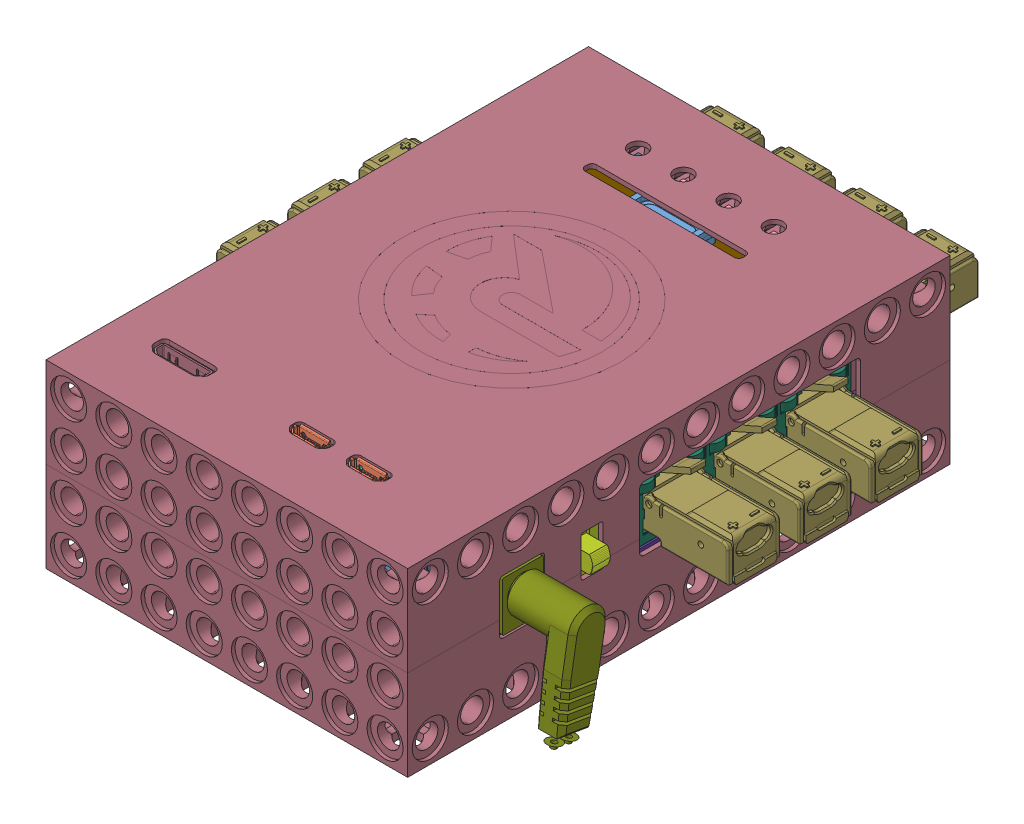
SolidWorks assembly PCBA_estimation_20190215, configuration Default. Lengths in mm.
Overall size (114.3 40.23 137.41).
1046 component instances, 72 part files, 0 mates.
Components (placement in the parent):
- RapberryPiZero-1: RapberryPiZero [Default] at (82.9427 2.6354 70.9883) x (1 0 0) z (0 1 0) size (66.85 4.45 31.23)
  - Raspberry_pizero_PCB-1: Raspberry_pizero_PCB [Default] at (-51.2564 20.0966 13.0542) size (65 1 30)
  - Micro USB_input_female (short)-SMT-1: Micro USB_input_female (short)-SMT [Default] at (-29.7564 22.3216 26.5042) size (7.98 2.94 5.43)
  - Micro USB_input_female (short)-SMT-2: Micro USB_input_female (short)-SMT [Default] at (-42.3564 22.3216 26.5042) size (7.98 2.94 5.43)
  - 0204 - Capacitor-1: 0204 - Capacitor [Default] at (-60.0807 21.3466 22.3712) x (0 0 -1) z (1 0 0) size (1.08 0.58 0.68)
  - 0204 - Capacitor-2: 0204 - Capacitor [Default] at (-43.6156 21.3466 13.1418) size (1.08 0.58 0.68)
  - 0204 - Capacitor-3: 0204 - Capacitor [Default] at (-62.4121 21.3466 11.2398) size (1.08 0.58 0.68)
  - 0204 - Capacitor-4: 0204 - Capacitor [Default] at (-45.7322 21.3466 20.0663) size (1.08 0.58 0.68)
  - 0204 - Capacitor-5: 0204 - Capacitor [Default] at (-43.6156 21.3466 10.1424) size (1.08 0.58 0.68)
  - 0204 - Capacitor-6: 0204 - Capacitor [Default] at (-59.0466 21.3466 22.3712) x (0 0 -1) z (1 0 0) size (1.08 0.58 0.68)
  - 0204 - Capacitor-7: 0204 - Capacitor [Default] at (-46.3457 21.3466 16.1412) size (1.08 0.58 0.68)
  - 0204 - Capacitor-8: 0204 - Capacitor [Default] at (-48.9117 21.3466 7.6917) size (1.08 0.58 0.68)
  - 0204 - Capacitor-9: 0204 - Capacitor [Default] at (-62.5919 21.3466 21.919) size (1.08 0.58 0.68)
  - 0204 - Capacitor-10: 0204 - Capacitor [Default] at (-48.1448 21.3466 22.316) x (0 0 -1) z (1 0 0) size (1.08 0.58 0.68)
  - 0204 - Capacitor-11: 0204 - Capacitor [Default] at (-55.4926 21.3466 7.2526) x (0 0 -1) z (1 0 0) size (1.08 0.58 0.68)
  - 0204 - Capacitor-12: 0204 - Capacitor [Default] at (-52.6496 21.3466 22.316) x (0 0 1) z (-1 0 0) size (1.08 0.58 0.68)
  - 0204 - Capacitor-13: 0204 - Capacitor [Default] at (-53.7932 21.3466 7.2526) x (0 0 1) z (-1 0 0) size (1.08 0.58 0.68)
  - 0204 - Capacitor-14: 0204 - Capacitor [Default] at (-61.8122 21.3466 17.2416) size (1.08 0.58 0.68)
  - 0204 - Capacitor-15: 0204 - Capacitor [Default] at (-45.7322 21.3466 19.0675) size (1.08 0.58 0.68)
  - 0204 - Capacitor-16: 0204 - Capacitor [Default] at (-60.4584 21.3466 22.3712) x (0 0 1) z (-1 0 0) size (1.08 0.58 0.68)
  - 0204 - Capacitor-17: 0204 - Capacitor [Default] at (-45.7322 21.3466 17.1095) size (1.08 0.58 0.68)
  - 0204 - Capacitor-18: 0204 - Capacitor [Default] at (-46.475 21.3466 21.113) size (1.08 0.58 0.68)
  - 0204 - Capacitor-19: 0204 - Capacitor [Default] at (-59.8477 21.3466 7.2526) x (0 0 1) z (-1 0 0) size (1.08 0.58 0.68)
  - 0204 - Capacitor-20: 0204 - Capacitor [Default] at (-46.3457 21.3466 15.1229) size (1.08 0.58 0.68)
  - 0204 - Capacitor-21: 0204 - Capacitor [Default] at (-45.7322 21.3466 18.1249) size (1.08 0.58 0.68)
  - 0204 - Capacitor-22: 0204 - Capacitor [Default] at (-51.2398 21.3466 22.316) x (0 0 -1) z (1 0 0) size (1.08 0.58 0.68)
  - 0204 - Capacitor-23: 0204 - Capacitor [Default] at (-47.1199 21.3466 23.926) x (0 0 1) z (-1 0 0) size (1.08 0.58 0.68)
  - 0204 - Capacitor-24: 0204 - Capacitor [Default] at (-62.4121 21.3466 12.2528) size (1.08 0.58 0.68)
  - 0204 - Capacitor-25: 0204 - Capacitor [Default] at (-48.9117 21.3466 6.5273) size (1.08 0.58 0.68)
  - 0204 - Capacitor-26: 0204 - Capacitor [Default] at (-61.8122 21.3466 13.3136) size (1.08 0.58 0.68)
  - 0204 - Capacitor-27: 0204 - Capacitor [Default] at (-61.8122 21.3466 15.241) size (1.08 0.58 0.68)
  - 0204 - Capacitor-28: 0204 - Capacitor [Default] at (-61.8122 21.3466 14.2646) size (1.08 0.58 0.68)
  - 0204 - Capacitor-29: 0204 - Capacitor [Default] at (-46.3457 21.3466 14.0197) size (1.08 0.58 0.68)
  - 0204 - Capacitor-30: 0204 - Capacitor [Default] at (-62.5919 21.3466 20.9695) size (1.08 0.58 0.68)
  - 0204 - Capacitor-31: 0204 - Capacitor [Default] at (-52.25 21.3466 22.316) x (0 0 -1) z (1 0 0) size (1.08 0.58 0.68)
  - 0204 - Capacitor-32: 0204 - Capacitor [Default] at (-61.8122 21.3466 16.2144) size (1.08 0.58 0.68)
  - 0204 - Capacitor-33: 0204 - Capacitor [Default] at (-46.3457 21.3466 12.9589) size (1.08 0.58 0.68)
  - 0204 - Capacitor-34: 0204 - Capacitor [Default] at (-49.1841 21.3466 22.316) x (0 0 -1) z (1 0 0) size (1.08 0.58 0.68)
  - 0204- Resistor-1: 0204- Resistor [Default] at (-61.8169 21.4522 19.8533) x (-1 0 0) z (0 -1 0) size (0.99 0.51 0.36)
  - 0204- Resistor-2: 0204- Resistor [Default] at (-43.6109 21.4522 15.4193) x (-1 0 0) z (0 -1 0) size (0.99 0.51 0.36)
  - 0204- Resistor-3: 0204- Resistor [Default] at (-65.0626 21.4522 16.5355) x (1 0 0) z (0 -1 0) size (0.99 0.51 0.36)
  - 0204- Resistor-4: 0204- Resistor [Default] at (-42.6936 21.4522 18.4076) x (-1 0 0) z (0 -1 0) size (0.99 0.51 0.36)
  - 0204- Resistor-5: 0204- Resistor [Default] at (-61.8169 21.4522 18.5178) x (-1 0 0) z (0 -1 0) size (0.99 0.51 0.36)
  - 0204- Resistor-6: 0204- Resistor [Default] at (-79.148 21.4522 17.7279) x (-1 0 0) z (0 -1 0) size (0.99 0.51 0.36)
  - 0204- Resistor-7: 0204- Resistor [Default] at (-39.831 21.4522 18.1462) x (0 0 1) z (0 -1 0) size (0.99 0.51 0.36)
  - 0204- Resistor-8: 0204- Resistor [Default] at (-78.9105 21.4522 21.1554) x (1 0 0) z (0 -1 0) size (0.99 0.51 0.36)
  - 0204- Resistor-9: 0204- Resistor [Default] at (-43.6109 21.4522 14.4127) x (-1 0 0) z (0 -1 0) size (0.99 0.51 0.36)
  - 0204- Resistor-10: 0204- Resistor [Default] at (-52.4165 21.4522 24.0419) x (1 0 0) z (0 -1 0) size (0.99 0.51 0.36)
  - 0204- Resistor-11: 0204- Resistor [Default] at (-43.6109 21.4522 12.4047) x (-1 0 0) z (0 -1 0) size (0.99 0.51 0.36)
  - 0204- Resistor-12: 0204- Resistor [Default] at (-68.4329 21.4522 5.4384) x (0 0 1) z (0 -1 0) size (0.99 0.51 0.36)
  - 0204- Resistor-13: 0204- Resistor [Default] at (-21.8613 21.4522 20.9026) x (-1 0 0) z (0 -1 0) size (0.99 0.51 0.36)
  - 0204- Resistor-14: 0204- Resistor [Default] at (-69.7255 21.4522 5.4384) x (0 0 1) z (0 -1 0) size (0.99 0.51 0.36)
  - 0204- Resistor-15: 0204- Resistor [Default] at (-56.0985 21.4522 7.2479) x (0 0 -1) z (0 -1 0) size (0.99 0.51 0.36)
  - 0204- Resistor-16: 0204- Resistor [Default] at (-48.8769 21.4522 23.8207) x (1 0 0) z (0 -1 0) size (0.99 0.51 0.36)
  - 0204- Resistor-17: 0204- Resistor [Default] at (-28.0827 21.4522 9.5819) x (-1 0 0) z (0 -1 0) size (0.99 0.51 0.36)
  - CAP-0306-1: CAP-0306 [Default] at (-45.8903 21.4966 8.7634) size (1.6 0.8 0.9)
  - CAP-0306-2: CAP-0306 [Default] at (-82.0031 21.4966 19.0464) x (0 0 1) z (-1 0 0) size (1.6 0.8 0.9)
  - Raspberry_pizero_BCM2835 with VC4-1: Raspberry_pizero_BCM2835 with VC4 [Default] at (-54.1608 21.5466 15.1238) x (1 0 0) z (0 0 -1) size (12 0.65 12)
  - Crystal 3.4x2.4mm-1: Crystal 3.4x2.4mm [Default] at (-65.3089 21.0966 19.2633) size (3.2 1 2.4)
  - 32,768 Khz Crystal-1: 32,768 Khz Crystal [Default] at (-60.5154 21.1428 26.5473) x (0.999848 -0.017452 0) z (0 0 1) size (3.4 1.03 1.5)
  - 0805- Capacitor-1: 0805- Capacitor [Default] at (-27.9052 21.9966 13.3538) x (0 0 -1) z (0 -1 0) size (2 1.25 0.9)
  - 0805- Capacitor-2: 0805- Capacitor [Default] at (-29.8247 21.9966 13.3538) x (0 0 1) z (0 -1 0) size (2 1.25 0.9)
  - 0805- Capacitor-3: 0805- Capacitor [Default] at (-20.9924 21.9966 13.3538) x (0 0 -1) z (0 -1 0) size (2 1.25 0.9)
  - 0805- Capacitor-4: 0805- Capacitor [Default] at (-51.9496 21.9966 7.3589) x (1 0 0) z (0 -1 0) size (2 1.25 0.9)
  - 0805- Capacitor-5: 0805- Capacitor [Default] at (-37.009 21.9966 22.5384) x (0 0 -1) z (0 -1 0) size (2 1.25 0.9)
  - 0805- Capacitor-6: 0805- Capacitor [Default] at (-51.9496 21.9966 5.2384) x (1 0 0) z (0 -1 0) size (2 1.25 0.9)
  - 0805- Capacitor-7: 0805- Capacitor [Default] at (-22.8003 21.9966 13.3538) x (0 0 -1) z (0 -1 0) size (2 1.25 0.9)
  - 0204 - Capacitor Brown-1: 0204 - Capacitor Brown [Default] at (-28.0874 21.3466 10.3236) size (1.08 0.58 0.68)
  - 0204 - Capacitor Brown-2: 0204 - Capacitor Brown [Default] at (-46.3457 21.3466 10.1566) size (1.08 0.58 0.68)
  - 0204 - Capacitor Brown-3: 0204 - Capacitor Brown [Default] at (-43.6156 21.3466 11.1151) size (1.08 0.58 0.68)
  - 0204 - Capacitor Brown-4: 0204 - Capacitor Brown [Default] at (-64.0312 21.3466 26.8794) size (1.08 0.58 0.68)
  - 0204 - Capacitor Brown-5: 0204 - Capacitor Brown [Default] at (-46.3457 21.3466 11.0963) size (1.08 0.58 0.68)
  - 0204 - Capacitor Brown-6: 0204 - Capacitor Brown [Default] at (-57.5817 21.3466 26.803) size (1.08 0.58 0.68)
  - 0204 - Capacitor Brown-7: 0204 - Capacitor Brown [Default] at (-46.3457 21.3466 12.214) size (1.08 0.58 0.68)
  - 0204 - Capacitor Brown-8: 0204 - Capacitor Brown [Default] at (-80.6197 21.3466 20.6997) size (1.08 0.58 0.68)
  - 6-Pin SOT-1: 6-Pin SOT [Default] at (-79.714 21.0966 19.2138) x (0 0 1) z (0 1 0) size (1.5 1.84 0.95)
  - micro sd molex-1: micro sd molex [Default] at (-74.7768 21.6766 -33.0961) x (0 0 1) z (0 1 0) size (11.95 11.4 1.45)
  - hdmi type C-1: hdmi type C [Default] at (-71.3564 22.9466 28.6542) size (12.9 4.05 7.7)
  - Voltage Regulator 3x3mm 12-Pin-1: Voltage Regulator 3x3mm 12-Pin [Default] at (-23.6842 21.0966 12.6105) x (1 0 0) z (0 1 0) size (3 4.1 1.28)
  - 1210 inductor-1: 1210 inductor [Default] at (-46.4963 21.0916 6.3909) x (0 0 1) z (0 1 0) size (3.43 2.77 0.72)
  - 1210 inductor-2: 1210 inductor [Default] at (-28.2854 21.0916 17.6682) x (1 0 0) z (0 1 0) size (3.43 2.77 0.72)
  - 1210 inductor-3: 1210 inductor [Default] at (-22.7405 21.0916 9.2394) x (1 0 0) z (0 1 0) size (3.43 2.77 0.72)
  - 545482271-1: 545482271 [Default] at (-21.4564 21.1166 13.0542) x (0 0 -1) z (1 0 0) size (16.2 1.2 5)
- RRRC_carrier_board-1: RRRC_carrier_board [Default] at (75.1836 8.28 47.3515) x (0 0 -1) z (0 1 0) size (102.74 81.4 21.81)
  - Board_CARRIER_3-1: Board_CARRIER_3 [Default] at origin size (102.7 77 1.61)
    - Open CASCADE STEP translator 6.8 1.1.1_2-1: Open CASCADE STEP translator 6.8 1.1.1_2 [Default] at (0 0 -1.61) size (102.7 77 1.61)
  - D59_CARRIER_3-1: D59_CARRIER_3 [Default] at origin size (0.65 1.05 0.44)
    - SOD-923_3-1: SOD-923_3 [Default] at (80 52.05 0) x (0 1 0) z (1 0 0) size (1.05 0.44 0.65)
  - D15_CARRIER_3-1: D15_CARRIER_3 [Default] at origin size (1.7 1.7 0.64)
    - SOT-666_3-1: SOT-666_3 [Default] at (15.825 38.45 0) x (1 0 0) z (0 0 1) size (1.7 1.7 0.64)
  - C71_CARRIER_3-1: C71_CARRIER_3 [Default] at origin size (1 0.5 0.5)
    - C_0402_3-1: C_0402_3 [Default] at (44.4 57.5 0) x (-1 0 0) z (0 0 1) size (1 0.5 0.5)
  - D71_CARRIER_3-1: D71_CARRIER_3 [Default] at origin size (1.05 0.65 0.44)
    - SOD-923_3-1: SOD-923_3 [Default] at (62.45 58.75 0) x (-1 0 0) z (0 1 0) size (1.05 0.44 0.65)
  - D70_CARRIER_3-1: D70_CARRIER_3 [Default] at origin size (1.05 0.65 0.44)
    - SOD-923_3-1: SOD-923_3 [Default] at (66.95 57.6 0) x (1 0 0) z (0 -1 0) size (1.05 0.44 0.65)
  - D69_CARRIER_3-1: D69_CARRIER_3 [Default] at origin size (1.05 0.65 0.44)
    - SOD-923_3-1: SOD-923_3 [Default] at (50.1 57.5 0) x (1 0 0) z (0 -1 0) size (1.05 0.44 0.65)
  - D68_CARRIER_3-1: D68_CARRIER_3 [Default] at origin size (1.05 0.65 0.44)
    - SOD-923_3-1: SOD-923_3 [Default] at (52.85 58.45 0) x (-1 0 0) z (0 1 0) size (1.05 0.44 0.65)
  - D67_CARRIER_3-1: D67_CARRIER_3 [Default] at origin size (1.05 0.65 0.44)
    - SOD-923_3-1: SOD-923_3 [Default] at (37.65 58.6 0) x (1 0 0) z (0 -1 0) size (1.05 0.44 0.65)
  - D66_CARRIER_3-1: D66_CARRIER_3 [Default] at origin size (1.05 0.65 0.44)
    - SOD-923_3-1: SOD-923_3 [Default] at (44.35 58.55 0) x (-1 0 0) z (0 1 0) size (1.05 0.44 0.65)
  - D65_CARRIER_3-1: D65_CARRIER_3 [Default] at origin size (1.05 0.65 0.44)
    - SOD-923_3-1: SOD-923_3 [Default] at (46.8 18.45 0) x (-1 0 0) z (0 1 0) size (1.05 0.44 0.65)
  - D64_CARRIER_3-1: D64_CARRIER_3 [Default] at origin size (1.05 0.65 0.44)
    - SOD-923_3-1: SOD-923_3 [Default] at (42.85 18.35 0) x (-1 0 0) z (0 1 0) size (1.05 0.44 0.65)
  - D63_CARRIER_3-1: D63_CARRIER_3 [Default] at origin size (1.05 0.65 0.44)
    - SOD-923_3-1: SOD-923_3 [Default] at (60.1 19.2 0) x (1 0 0) z (0 -1 0) size (1.05 0.44 0.65)
  - D62_CARRIER_3-1: D62_CARRIER_3 [Default] at origin size (1.05 0.65 0.44)
    - SOD-923_3-1: SOD-923_3 [Default] at (56.05 18.45 0) x (-1 0 0) z (0 1 0) size (1.05 0.44 0.65)
  - D61_CARRIER_3-1: D61_CARRIER_3 [Default] at origin size (1.05 0.65 0.44)
    - SOD-923_3-1: SOD-923_3 [Default] at (73.3 18.5 0) x (-1 0 0) z (0 1 0) size (1.05 0.44 0.65)
  - D60_CARRIER_3-1: D60_CARRIER_3 [Default] at origin size (1.05 0.65 0.44)
    - SOD-923_3-1: SOD-923_3 [Default] at (69.4 18.5 0) x (-1 0 0) z (0 1 0) size (1.05 0.44 0.65)
  - D11_CARRIER_3-1: D11_CARRIER_3 [Default] at origin size (1.15 0.55 0.41)
    - R_0402_3-1: R_0402_3 [Default] at (48.775 25.425 0) x (1 0 0) z (0 -1 0) size (1.15 0.41 0.55)
  - R99_CARRIER_3-1: R99_CARRIER_3 [Default] at origin size (1.15 0.55 0.41)
    - R_0402_3-1: R_0402_3 [Default] at (83.975 18.15 0) x (-1 0 0) z (0 1 0) size (1.15 0.41 0.55)
  - D58_CARRIER_3-1: D58_CARRIER_3 [Default] at origin size (1.05 0.65 0.44)
    - SOD-923_3-1: SOD-923_3 [Default] at (78.05 20.3 0) x (-1 0 0) z (0 1 0) size (1.05 0.44 0.65)
  - D57_CARRIER_3-1: D57_CARRIER_3 [Default] at origin size (0.65 1.05 0.44)
    - SOD-923_3-1: SOD-923_3 [Default] at (79.85 30.3 0) x (0 1 0) z (1 0 0) size (1.05 0.44 0.65)
  - D56_CARRIER_3-1: D56_CARRIER_3 [Default] at origin size (0.65 1.05 0.44)
    - SOD-923_3-1: SOD-923_3 [Default] at (79.7 41.4 0) x (0 1 0) z (1 0 0) size (1.05 0.44 0.65)
  - R160_CARRIER_3-1: R160_CARRIER_3 [Default] at origin size (1.15 0.55 0.41)
    - R_0402_3-1: R_0402_3 [Default] at (2.375 14.45 0) x (1 0 0) z (0 -1 0) size (1.15 0.41 0.55)
  - R159_CARRIER_3-1: R159_CARRIER_3 [Default] at origin size (1.15 0.55 0.41)
    - R_0402_3-1: R_0402_3 [Default] at (2.375 15.5 0) x (1 0 0) z (0 -1 0) size (1.15 0.41 0.55)
  - R158_CARRIER_3-1: R158_CARRIER_3 [Default] at origin size (0.55 1.15 0.41)
    - R_0402_3-1: R_0402_3 [Default] at (9.4 16 0) x (0 -1 0) z (-1 0 0) size (1.15 0.41 0.55)
  - Q19_CARRIER_3-1: Q19_CARRIER_3 [Default] at origin size (3.05 3 1.41)
    - SOT95P255X140-3N_3-1: SOT95P255X140-3N_3 [Default] at (5.9 15.45 0) x (0 1 0) z (0 0 1) size (3 3.05 1.41)
  - D24_CARRIER_3-1: D24_CARRIER_3 [Default] at origin size (1.05 0.65 0.44)
    - SOD-923_3-1: SOD-923_3 [Default] at (82.6 28.05 0) x (-1 0 0) z (0 1 0) size (1.05 0.44 0.65)
  - CON1_CARRIER_3-1: CON1_CARRIER_3 [Default] at origin size (6.35 2.14 6.3)
    - SULLINS_GRPB051VWVN-RC_3-1: SULLINS_GRPB051VWVN-RC_3 [Default] at (60.4749 35.8 0) x (1 0 0) z (0 -1 0) size (6.35 6.3 2.14)
  - D54_CARRIER_3-1: D54_CARRIER_3 [Default] at origin size (1.6 3.6 1.3)
    - SOD360X160X130L37X85N_3-1: SOD360X160X130L37X85N_3 [Default] at (57.2 45.75 0) x (0 1 0) z (0 0 1) size (3.6 1.6 1.3)
  - D55_CARRIER_3-1: D55_CARRIER_3 [Default] at origin size (1.6 3.6 1.3)
    - SOD360X160X130L37X85N_3-1: SOD360X160X130L37X85N_3 [Default] at (51.35 45.6 0) x (0 1 0) z (0 0 1) size (3.6 1.6 1.3)
  - Q17_CARRIER_3-1: Q17_CARRIER_3 [Default] at origin size (3.05 3 1.41)
    - SOT95P255X140-3N_3-1: SOT95P255X140-3N_3 [Default] at (54.3 45.7 0) x (0 1 0) z (0 0 1) size (3 3.05 1.41)
  - Q18_CARRIER_3-1: Q18_CARRIER_3 [Default] at origin size (3.05 3 1.41)
    - SOT95P255X140-3N_3-1: SOT95P255X140-3N_3 [Default] at (48.43 45.65 0) x (0 1 0) z (0 0 1) size (3 3.05 1.41)
  - R142_CARRIER_3-1: R142_CARRIER_3 [Default] at origin size (1.15 0.55 0.41)
    - R_0402_3-1: R_0402_3 [Default] at (43.65 48 0) x (-1 0 0) z (0 1 0) size (1.15 0.41 0.55)
  - R144_CARRIER_3-1: R144_CARRIER_3 [Default] at origin size (1.15 0.55 0.41)
    - R_0402_3-1: R_0402_3 [Default] at (49.55 48.1 0) x (1 0 0) z (0 -1 0) size (1.15 0.41 0.55)
  - R147_CARRIER_3-1: R147_CARRIER_3 [Default] at origin size (1.15 0.55 0.41)
    - R_0402_3-1: R_0402_3 [Default] at (48.2 43.2 0) x (-1 0 0) z (0 1 0) size (1.15 0.41 0.55)
  - R139_CARRIER_3-1: R139_CARRIER_3 [Default] at origin size (1.15 0.55 0.41)
    - R_0402_3-1: R_0402_3 [Default] at (48.05 37.2 0) x (-1 0 0) z (0 1 0) size (1.15 0.41 0.55)
  - R135_CARRIER_3-1: R135_CARRIER_3 [Default] at origin size (1.15 0.55 0.41)
    - R_0402_3-1: R_0402_3 [Default] at (48.975 42.1 0) x (1 0 0) z (0 -1 0) size (1.15 0.41 0.55)
  - R133_CARRIER_3-1: R133_CARRIER_3 [Default] at origin size (1.15 0.55 0.41)
    - R_0402_3-1: R_0402_3 [Default] at (43.7 42.15 0) x (-1 0 0) z (0 1 0) size (1.15 0.41 0.55)
  - Q16_CARRIER_3-1: Q16_CARRIER_3 [Default] at origin size (3.05 3 1.41)
    - SOT95P255X140-3N_3-1: SOT95P255X140-3N_3 [Default] at (48.5 39.65 0) x (0 1 0) z (0 0 1) size (3 3.05 1.41)
  - Q15_CARRIER_3-1: Q15_CARRIER_3 [Default] at origin size (3.05 3 1.41)
    - SOT95P255X140-3N_3-1: SOT95P255X140-3N_3 [Default] at (54.35 39.65 0) x (0 1 0) z (0 0 1) size (3 3.05 1.41)
  - D53_CARRIER_3-1: D53_CARRIER_3 [Default] at origin size (1.6 3.6 1.3)
    - SOD360X160X130L37X85N_3-1: SOD360X160X130L37X85N_3 [Default] at (51.425 39.7 0) x (0 1 0) z (0 0 1) size (3.6 1.6 1.3)
  - D52_CARRIER_3-1: D52_CARRIER_3 [Default] at origin size (1.6 3.6 1.3)
    - SOD360X160X130L37X85N_3-1: SOD360X160X130L37X85N_3 [Default] at (57.25 39.7 0) x (0 1 0) z (0 0 1) size (3.6 1.6 1.3)
  - D50_CARRIER_3-1: D50_CARRIER_3 [Default] at origin size (1.6 3.6 1.3)
    - SOD360X160X130L37X85N_3-1: SOD360X160X130L37X85N_3 [Default] at (45.6278 39.7 0) x (0 1 0) z (0 0 1) size (3.6 1.6 1.3)
  - D51_CARRIER_3-1: D51_CARRIER_3 [Default] at origin size (1.6 3.6 1.3)
    - SOD360X160X130L37X85N_3-1: SOD360X160X130L37X85N_3 [Default] at (39.825 39.675 0) x (0 1 0) z (0 0 1) size (3.6 1.6 1.3)
  - Q13_CARRIER_3-1: Q13_CARRIER_3 [Default] at origin size (3.05 3 1.41)
    - SOT95P255X140-3N_3-1: SOT95P255X140-3N_3 [Default] at (42.725 39.65 0) x (0 1 0) z (0 0 1) size (3 3.05 1.41)
  - Q14_CARRIER_3-1: Q14_CARRIER_3 [Default] at origin size (3.05 3 1.41)
    - SOT95P255X140-3N_3-1: SOT95P255X140-3N_3 [Default] at (36.95 39.55 0) x (0 1 0) z (0 0 1) size (3 3.05 1.41)
  - R126_CARRIER_3-1: R126_CARRIER_3 [Default] at origin size (1.15 0.55 0.41)
    - R_0402_3-1: R_0402_3 [Default] at (41.65 42.15 0) x (1 0 0) z (0 -1 0) size (1.15 0.41 0.55)
  - R127_CARRIER_3-1: R127_CARRIER_3 [Default] at origin size (1.15 0.55 0.41)
    - R_0402_3-1: R_0402_3 [Default] at (37.525 42 0) x (1 0 0) z (0 -1 0) size (1.15 0.41 0.55)
  - R132_CARRIER_3-1: R132_CARRIER_3 [Default] at origin size (1.15 0.55 0.41)
    - R_0402_3-1: R_0402_3 [Default] at (37.75 37.1 0) x (-1 0 0) z (0 1 0) size (1.15 0.41 0.55)
  - CON9_CARRIER_2-1: CON9_CARRIER_2 [Default] at origin size (7 3.6 4.32)
    - BM05B-SRSS-TB_2-1: BM05B-SRSS-TB_2 [Default] at (38.7999 30.2499 0.025) x (-1 0 0) z (0 1 0) size (7 4.32 3.6)
  - C42_CARRIER_3-1: C42_CARRIER_3 [Default] at origin size (3.2 1.6 1.6)
    - C_1206_3-1: C_1206_3 [Default] at (58.5 25.4 0) x (1 0 0) z (0 0 1) size (3.2 1.6 1.6)
  - C39_CARRIER_3-1: C39_CARRIER_3 [Default] at origin size (3.2 1.6 1.6)
    - C_1206_3-1: C_1206_3 [Default] at (72.15 25.475 0) x (1 0 0) z (0 0 1) size (3.2 1.6 1.6)
  - C33_CARRIER_3-1: C33_CARRIER_3 [Default] at origin size (1 0.5 0.5)
    - C_0402_3-1: C_0402_3 [Default] at (59.5 46.5 0) x (1 0 0) z (0 0 1) size (1 0.5 0.5)
  - C36_CARRIER_3-1: C36_CARRIER_3 [Default] at origin size (1 0.5 0.5)
    - C_0402_3-1: C_0402_3 [Default] at (64.95 38.65 0) x (1 0 0) z (0 0 1) size (1 0.5 0.5)
  - C86_CARRIER_3-1: C86_CARRIER_3 [Default] at origin size (1.6 3.2 1.6)
    - C_1206_3-1: C_1206_3 [Default] at (59.65 43.3 0) x (0 -1 0) z (0 0 1) size (3.2 1.6 1.6)
  - C90_CARRIER_3-1: C90_CARRIER_3 [Default] at origin size (1.6 3.2 1.6)
    - C_1206_3-1: C_1206_3 [Default] at (60.275 33.85 0) x (0 1 0) z (0 0 1) size (3.2 1.6 1.6)
  - D37_CARRIER_3-1: D37_CARRIER_3 [Default] at origin size (1.15 0.55 0.41)
    - R_0402_3-1: R_0402_3 [Default] at (61.6 48.95 0) x (1 0 0) z (0 -1 0) size (1.15 0.41 0.55)
  - D38_CARRIER_3-1: D38_CARRIER_3 [Default] at origin size (1.15 0.55 0.41)
    - R_0402_3-1: R_0402_3 [Default] at (63.6 48.95 0) x (-1 0 0) z (0 1 0) size (1.15 0.41 0.55)
  - D42_CARRIER_3-1: D42_CARRIER_3 [Default] at origin size (1.15 0.55 0.41)
    - R_0402_3-1: R_0402_3 [Default] at (67.675 48.95 0) x (-1 0 0) z (0 1 0) size (1.15 0.41 0.55)
  - D43_CARRIER_3-1: D43_CARRIER_3 [Default] at origin size (1.15 0.55 0.41)
    - R_0402_3-1: R_0402_3 [Default] at (65.675 48.95 0) x (1 0 0) z (0 -1 0) size (1.15 0.41 0.55)
  - U16_CARRIER_3-1: U16_CARRIER_3 [Default] at origin size (7.8 7.6 1.6)
    - TSSOP-24[12-12]_0.45_0.65_5.6x7.8x1.6_3-1: TSSOP-24[12-12]_0.45_0.65_5.6x7.8x1.6_3 [Default] at (64.6501 43.8499 0) x (-1 0 0) z (0 0 1) size (7.8 7.6 1.6)
  - R32_CARRIER_3-1: R32_CARRIER_3 [Default] at origin size (1.15 0.55 0.41)
    - R_0402_3-1: R_0402_3 [Default] at (48.9 59.5 0) x (1 0 0) z (0 -1 0) size (1.15 0.41 0.55)
  - R40_CARRIER_3-1: R40_CARRIER_3 [Default] at origin size (1.15 0.55 0.41)
    - R_0402_3-1: R_0402_3 [Default] at (47.05 54.4 0) x (1 0 0) z (0 -1 0) size (1.15 0.41 0.55)
  - R38_CARRIER_3-1: R38_CARRIER_3 [Default] at origin size (1.15 0.55 0.41)
    - R_0402_3-1: R_0402_3 [Default] at (44.4 59.55 0) x (1 0 0) z (0 -1 0) size (1.15 0.41 0.55)
  - R37_CARRIER_3-1: R37_CARRIER_3 [Default] at origin size (1.15 0.55 0.41)
    - R_0402_3-1: R_0402_3 [Default] at (37.65 59.6 0) x (-1 0 0) z (0 1 0) size (1.15 0.41 0.55)
  - R35_CARRIER_3-1: R35_CARRIER_3 [Default] at origin size (1.15 0.55 0.41)
    - R_0402_3-1: R_0402_3 [Default] at (38.2 56.35 0) x (-1 0 0) z (0 1 0) size (1.15 0.41 0.55)
  - R34_CARRIER_3-1: R34_CARRIER_3 [Default] at origin size (1.15 0.55 0.41)
    - R_0402_3-1: R_0402_3 [Default] at (44.4 56.45 0) x (1 0 0) z (0 -1 0) size (1.15 0.41 0.55)
  - R33_CARRIER_3-1: R33_CARRIER_3 [Default] at origin size (1.15 0.55 0.41)
    - R_0402_3-1: R_0402_3 [Default] at (45.05 54.4 0) x (1 0 0) z (0 -1 0) size (1.15 0.41 0.55)
  - R31_CARRIER_3-1: R31_CARRIER_3 [Default] at origin size (0.55 1.15 0.41)
    - R_0402_3-1: R_0402_3 [Default] at (39.2095 59.1056 0) x (0 1 0) z (1 0 0) size (1.15 0.41 0.55)
  - Q5_CARRIER_3-1: Q5_CARRIER_3 [Default] at origin size (3.05 3 1.41)
    - SOT95P255X140-3N_3-1: SOT95P255X140-3N_3 [Default] at (47.2 56.9 0) x (0 1 0) z (0 0 1) size (3 3.05 1.41)
  - FU8_CARRIER_3-1: FU8_CARRIER_3 [Default] at origin size (1.5 2.3 1.25)
    - BELFUSE_0ZCK_3-1: BELFUSE_0ZCK_3 [Default] at (42.45 58.35 0) x (0 1 0) z (1 0 0) size (2.3 1.25 1.5)
  - FU7_CARRIER_3-1: FU7_CARRIER_3 [Default] at origin size (1.5 2.3 1.25)
    - BELFUSE_0ZCK_3-1: BELFUSE_0ZCK_3 [Default] at (40.616 58.3539 0) x (0 1 0) z (1 0 0) size (2.3 1.25 1.5)
  - D36_CARRIER_3-1: D36_CARRIER_3 [Default] at origin size (1.05 0.65 0.44)
    - SOD-923_3-1: SOD-923_3 [Default] at (39.6 55.3 0) x (1 0 0) z (0 -1 0) size (1.05 0.44 0.65)
  - D35_CARRIER_3-1: D35_CARRIER_3 [Default] at origin size (1.05 0.65 0.44)
    - SOD-923_3-1: SOD-923_3 [Default] at (42.45 56 0) x (1 0 0) z (0 -1 0) size (1.05 0.44 0.65)
  - D34_CARRIER_3-1: D34_CARRIER_3 [Default] at origin size (1.05 0.65 0.44)
    - SOD-923_3-1: SOD-923_3 [Default] at (46.85 59.5 0) x (-1 0 0) z (0 1 0) size (1.05 0.44 0.65)
  - C63_CARRIER_3-1: C63_CARRIER_3 [Default] at origin size (1 0.5 0.5)
    - C_0402_3-1: C_0402_3 [Default] at (37.7 57.55 0) x (1 0 0) z (0 0 1) size (1 0.5 0.5)
  - C37_CARRIER_3-1: C37_CARRIER_3 [Default] at origin size (2 1.2 1.2)
    - C_0805_3-1: C_0805_3 [Default] at (39.15 53.85 0.1) x (1 0 0) z (0 0 1) size (2 1.2 1.2)
  - C35_CARRIER_3-1: C35_CARRIER_3 [Default] at origin size (1 0.5 0.5)
    - C_0402_3-1: C_0402_3 [Default] at (42.45 54.855 0) x (1 0 0) z (0 0 1) size (1 0.5 0.5)
  - C75_CARRIER_3-1: C75_CARRIER_3 [Default] at origin size (1 0.5 0.5)
    - C_0402_3-1: C_0402_3 [Default] at (56.85 54.9 0) x (1 0 0) z (0 0 1) size (1 0.5 0.5)
  - C77_CARRIER_3-1: C77_CARRIER_3 [Default] at origin size (2 1.2 1.2)
    - C_0805_3-1: C_0805_3 [Default] at (54.05 54.35 0.1) x (-1 0 0) z (0 0 1) size (2 1.2 1.2)
  - C79_CARRIER_3-1: C79_CARRIER_3 [Default] at origin size (1 0.5 0.5)
    - C_0402_3-1: C_0402_3 [Default] at (50 56.45 0) x (1 0 0) z (0 0 1) size (1 0.5 0.5)
  - C81_CARRIER_3-1: C81_CARRIER_3 [Default] at origin size (1 0.5 0.5)
    - C_0402_3-1: C_0402_3 [Default] at (53.05 57.45 0) x (-1 0 0) z (0 0 1) size (1 0.5 0.5)
  - D39_CARRIER_3-1: D39_CARRIER_3 [Default] at origin size (1.05 0.65 0.44)
    - SOD-923_3-1: SOD-923_3 [Default] at (60.6 59.5 0) x (-1 0 0) z (0 1 0) size (1.05 0.44 0.65)
  - D40_CARRIER_3-1: D40_CARRIER_3 [Default] at origin size (1.05 0.65 0.44)
    - SOD-923_3-1: SOD-923_3 [Default] at (56.95 55.9 0) x (1 0 0) z (0 -1 0) size (1.05 0.44 0.65)
  - D41_CARRIER_3-1: D41_CARRIER_3 [Default] at origin size (1.05 0.65 0.44)
    - SOD-923_3-1: SOD-923_3 [Default] at (55 55.9 0) x (-1 0 0) z (0 1 0) size (1.05 0.44 0.65)
  - FU10_CARRIER_3-1: FU10_CARRIER_3 [Default] at origin size (1.5 2.3 1.25)
    - BELFUSE_0ZCK_3-1: BELFUSE_0ZCK_3 [Default] at (56.8 58.25 0) x (0 1 0) z (1 0 0) size (2.3 1.25 1.5)
  - FU9_CARRIER_3-1: FU9_CARRIER_3 [Default] at origin size (1.5 2.3 1.25)
    - BELFUSE_0ZCK_3-1: BELFUSE_0ZCK_3 [Default] at (55 58.25 0) x (0 1 0) z (1 0 0) size (2.3 1.25 1.5)
  - Q6_CARRIER_3-1: Q6_CARRIER_3 [Default] at origin size (3.05 3 1.41)
    - SOT95P255X140-3N_3-1: SOT95P255X140-3N_3 [Default] at (59.625 57 0) x (0 1 0) z (0 0 1) size (3 3.05 1.41)
  - R36_CARRIER_3-1: R36_CARRIER_3 [Default] at origin size (1.15 0.55 0.41)
    - R_0402_3-1: R_0402_3 [Default] at (53.05 59.5 0) x (1 0 0) z (0 -1 0) size (1.15 0.41 0.55)
  - R39_CARRIER_3-1: R39_CARRIER_3 [Default] at origin size (0.55 1.15 0.41)
    - R_0402_3-1: R_0402_3 [Default] at (66.4 59.15 0) x (0 1 0) z (1 0 0) size (1.15 0.41 0.55)
  - R42_CARRIER_3-1: R42_CARRIER_3 [Default] at origin size (1.15 0.55 0.41)
    - R_0402_3-1: R_0402_3 [Default] at (59.4 54.55 0) x (1 0 0) z (0 -1 0) size (1.15 0.41 0.55)
  - R43_CARRIER_3-1: R43_CARRIER_3 [Default] at origin size (1.15 0.55 0.41)
    - R_0402_3-1: R_0402_3 [Default] at (53.1 56.4 0) x (1 0 0) z (0 -1 0) size (1.15 0.41 0.55)
  - R44_CARRIER_3-1: R44_CARRIER_3 [Default] at origin size (0.55 1.15 0.41)
    - R_0402_3-1: R_0402_3 [Default] at (51.5 56.95 0) x (0 -1 0) z (-1 0 0) size (1.15 0.41 0.55)
  - R46_CARRIER_3-1: R46_CARRIER_3 [Default] at origin size (0.55 1.15 0.41)
    - R_0402_3-1: R_0402_3 [Default] at (50.45 59 0) x (0 1 0) z (1 0 0) size (1.15 0.41 0.55)
  - R47_CARRIER_3-1: R47_CARRIER_3 [Default] at origin size (0.55 1.15 0.41)
    - R_0402_3-1: R_0402_3 [Default] at (51.5 59 0) x (0 1 0) z (1 0 0) size (1.15 0.41 0.55)
  - R48_CARRIER_3-1: R48_CARRIER_3 [Default] at origin size (1.15 0.55 0.41)
    - R_0402_3-1: R_0402_3 [Default] at (58.75 59.5 0) x (-1 0 0) z (0 1 0) size (1.15 0.41 0.55)
  - C32_CARRIER_3-1: C32_CARRIER_3 [Default] at origin size (0.5 1 0.5)
    - C_0402_3-1: C_0402_3 [Default] at (33.2 7.8 0) x (0 1 0) z (0 0 1) size (1 0.5 0.5)
  - C24_CARRIER_3-1: C24_CARRIER_3 [Default] at origin size (0.5 1 0.5)
    - C_0402_3-1: C_0402_3 [Default] at (58.6 35.2 0) x (0 1 0) z (0 0 1) size (1 0.5 0.5)
  - C28_CARRIER_3-1: C28_CARRIER_3 [Default] at origin size (1 0.5 0.5)
    - C_0402_3-1: C_0402_3 [Default] at (51.45 35.775 0) x (-1 0 0) z (0 0 1) size (1 0.5 0.5)
  - C34_CARRIER_3-1: C34_CARRIER_3 [Default] at origin size (1.6 3.2 1.6)
    - C_1206_3-1: C_1206_3 [Default] at (57 33.7 0) x (0 1 0) z (0 0 1) size (3.2 1.6 1.6)
  - C73_CARRIER_3-1: C73_CARRIER_3 [Default] at origin size (1.6 3.2 1.6)
    - C_1206_3-1: C_1206_3 [Default] at (46.5 34.1 0) x (0 1 0) z (0 0 1) size (3.2 1.6 1.6)
  - D31_CARRIER_3-1: D31_CARRIER_3 [Default] at origin size (1.15 0.55 0.41)
    - R_0402_3-1: R_0402_3 [Default] at (50.775 25.425 0) x (-1 0 0) z (0 1 0) size (1.15 0.41 0.55)
  - D32_CARRIER_3-1: D32_CARRIER_3 [Default] at origin size (1.15 0.55 0.41)
    - R_0402_3-1: R_0402_3 [Default] at (54.85 25.425 0) x (-1 0 0) z (0 1 0) size (1.15 0.41 0.55)
  - D33_CARRIER_3-1: D33_CARRIER_3 [Default] at origin size (1.15 0.55 0.41)
    - R_0402_3-1: R_0402_3 [Default] at (52.85 25.425 0) x (1 0 0) z (0 -1 0) size (1.15 0.41 0.55)
  - U15_CARRIER_3-1: U15_CARRIER_3 [Default] at origin size (7.8 7.6 1.6)
    - TSSOP-24[12-12]_0.45_0.65_5.6x7.8x1.6_3-1: TSSOP-24[12-12]_0.45_0.65_5.6x7.8x1.6_3 [Default] at (51.7999 30.5501 0) x (1 0 0) z (0 0 1) size (7.8 7.6 1.6)
  - U5_CARRIER_3-1: U5_CARRIER_3 [Default] at origin size (3 3.1 0.8)
    - DFN-6(3x3)_0.45_0.95_3x3x1_HD[2,50x1,75]_3-1: DFN-6(3x3)_0.45_0.95_3x3x1_HD[2,50x1,75]_3 [Default] at (45.125 28.675 0.05) x (0 1 0) z (0 0 1) size (3.1 3 0.8)
  - R29_CARRIER_3-1: R29_CARRIER_3 [Default] at origin size (1.15 0.55 0.41)
    - R_0402_3-1: R_0402_3 [Default] at (42.8 17.3 0) x (1 0 0) z (0 -1 0) size (1.15 0.41 0.55)
  - R28_CARRIER_3-1: R28_CARRIER_3 [Default] at origin size (1.15 0.55 0.41)
    - R_0402_3-1: R_0402_3 [Default] at (46.85 17.35 0) x (1 0 0) z (0 -1 0) size (1.15 0.41 0.55)
  - R24_CARRIER_3-1: R24_CARRIER_3 [Default] at origin size (0.55 1.15 0.41)
    - R_0402_3-1: R_0402_3 [Default] at (40.1 23.2 0) x (0 -1 0) z (-1 0 0) size (1.15 0.41 0.55)
  - R30_CARRIER_3-1: R30_CARRIER_3 [Default] at origin size (1.15 0.55 0.41)
    - R_0402_3-1: R_0402_3 [Default] at (41.65 22.7 0) x (-1 0 0) z (0 1 0) size (1.15 0.41 0.55)
  - Q4_CARRIER_3-1: Q4_CARRIER_3 [Default] at origin size (3.05 3 1.41)
    - SOT95P255X140-3N_3-1: SOT95P255X140-3N_3 [Default] at (39.75 19.825 0) x (0 -1 0) z (0 0 1) size (3 3.05 1.41)
  - FU6_CARRIER_3-1: FU6_CARRIER_3 [Default] at origin size (1.5 2.3 1.25)
    - BELFUSE_0ZCK_3-1: BELFUSE_0ZCK_3 [Default] at (44.85 19 0) x (0 -1 0) z (-1 0 0) size (2.3 1.25 1.5)
  - FU5_CARRIER_3-1: FU5_CARRIER_3 [Default] at origin size (1.5 2.3 1.25)
    - BELFUSE_0ZCK_3-1: BELFUSE_0ZCK_3 [Default] at (48.8 18.65 0) x (0 -1 0) z (-1 0 0) size (2.3 1.25 1.5)
  - D14_CARRIER_3-1: D14_CARRIER_3 [Default] at origin size (1.05 0.65 0.44)
    - SOD-923_3-1: SOD-923_3 [Default] at (49.4 22.95 0) x (-1 0 0) z (0 1 0) size (1.05 0.44 0.65)
  - D13_CARRIER_3-1: D13_CARRIER_3 [Default] at origin size (1.05 0.65 0.44)
    - SOD-923_3-1: SOD-923_3 [Default] at (44.3 21.55 0) x (1 0 0) z (0 -1 0) size (1.05 0.44 0.65)
  - D12_CARRIER_3-1: D12_CARRIER_3 [Default] at origin size (1.05 0.65 0.44)
    - SOD-923_3-1: SOD-923_3 [Default] at (40.55 17.375 0) x (-1 0 0) z (0 1 0) size (1.05 0.44 0.65)
  - C46_CARRIER_3-1: C46_CARRIER_3 [Default] at origin size (3.2 1.6 1.6)
    - C_1206_3-1: C_1206_3 [Default] at (44.15 25.35 0) x (1 0 0) z (0 0 1) size (3.2 1.6 1.6)
  - C53_CARRIER_3-1: C53_CARRIER_3 [Default] at origin size (1 0.5 0.5)
    - C_0402_3-1: C_0402_3 [Default] at (58.45 53.4 0) x (-1 0 0) z (0 0 1) size (1 0.5 0.5)
  - C31_CARRIER_3-1: C31_CARRIER_3 [Default] at origin size (1 0.5 0.5)
    - C_0402_3-1: C_0402_3 [Default] at (42.8 19.5 0) x (-1 0 0) z (0 0 1) size (1 0.5 0.5)
  - C30_CARRIER_3-1: C30_CARRIER_3 [Default] at origin size (1 0.5 0.5)
    - C_0402_3-1: C_0402_3 [Default] at (46.85 19.5 0) x (-1 0 0) z (0 0 1) size (1 0.5 0.5)
  - C27_CARRIER_3-1: C27_CARRIER_3 [Default] at origin size (1 0.5 0.5)
    - C_0402_3-1: C_0402_3 [Default] at (44.3 22.7 0) x (1 0 0) z (0 0 1) size (1 0.5 0.5)
  - C29_CARRIER_3-1: C29_CARRIER_3 [Default] at origin size (2 1.2 1.2)
    - C_0805_3-1: C_0805_3 [Default] at (49.6 21.375 0.1) x (-1 0 0) z (0 0 1) size (2 1.2 1.2)
  - R25_CARRIER_3-1: R25_CARRIER_3 [Default] at origin size (0.55 1.15 0.41)
    - R_0402_3-1: R_0402_3 [Default] at (42.275 21.025 0) x (0 1 0) z (1 0 0) size (1.15 0.41 0.55)
  - R26_CARRIER_3-1: R26_CARRIER_3 [Default] at origin size (0.55 1.15 0.41)
    - R_0402_3-1: R_0402_3 [Default] at (46.425 21.4 0) x (0 1 0) z (1 0 0) size (1.15 0.41 0.55)
  - R18_CARRIER_3-1: R18_CARRIER_3 [Default] at origin size (1.15 0.55 0.41)
    - R_0402_3-1: R_0402_3 [Default] at (60.1 21.2 0) x (-1 0 0) z (0 1 0) size (1.15 0.41 0.55)
  - R17_CARRIER_3-1: R17_CARRIER_3 [Default] at origin size (0.55 1.15 0.41)
    - R_0402_3-1: R_0402_3 [Default] at (55.55 20.95 0) x (0 1 0) z (1 0 0) size (1.15 0.41 0.55)
  - C21_CARRIER_3-1: C21_CARRIER_3 [Default] at origin size (2 1.2 1.2)
    - C_0805_3-1: C_0805_3 [Default] at (62.9 21.3 0.1) x (-1 0 0) z (0 0 1) size (2 1.2 1.2)
  - C19_CARRIER_3-1: C19_CARRIER_3 [Default] at origin size (1 0.5 0.5)
    - C_0402_3-1: C_0402_3 [Default] at (57.6 22.65 0) x (1 0 0) z (0 0 1) size (1 0.5 0.5)
  - C23_CARRIER_3-1: C23_CARRIER_3 [Default] at origin size (1 0.5 0.5)
    - C_0402_3-1: C_0402_3 [Default] at (60.1 20.2 0) x (1 0 0) z (0 0 1) size (1 0.5 0.5)
  - C25_CARRIER_3-1: C25_CARRIER_3 [Default] at origin size (1 0.5 0.5)
    - C_0402_3-1: C_0402_3 [Default] at (56.075 19.45 0) x (-1 0 0) z (0 0 1) size (1 0.5 0.5)
  - C49_CARRIER_3-1: C49_CARRIER_3 [Default] at origin size (1 0.5 0.5)
    - C_0402_3-1: C_0402_3 [Default] at (46.95 49.2 0) x (1 0 0) z (0 0 1) size (1 0.5 0.5)
  - C51_CARRIER_3-1: C51_CARRIER_3 [Default] at origin size (1 0.5 0.5)
    - C_0402_3-1: C_0402_3 [Default] at (55.2 49.3 0) x (1 0 0) z (0 0 1) size (1 0.5 0.5)
  - D10_CARRIER_3-1: D10_CARRIER_3 [Default] at origin size (1.05 0.65 0.44)
    - SOD-923_3-1: SOD-923_3 [Default] at (62.35 23 0) x (-1 0 0) z (0 1 0) size (1.05 0.44 0.65)
  - D8_CARRIER_3-1: D8_CARRIER_3 [Default] at origin size (1.05 0.65 0.44)
    - SOD-923_3-1: SOD-923_3 [Default] at (53.875 17.4 0) x (-1 0 0) z (0 1 0) size (1.05 0.44 0.65)
  - D9_CARRIER_3-1: D9_CARRIER_3 [Default] at origin size (1.05 0.65 0.44)
    - SOD-923_3-1: SOD-923_3 [Default] at (57.6 21.5 0) x (1 0 0) z (0 -1 0) size (1.05 0.44 0.65)
  - FU3_CARRIER_3-1: FU3_CARRIER_3 [Default] at origin size (1.5 2.3 1.25)
    - BELFUSE_0ZCK_3-1: BELFUSE_0ZCK_3 [Default] at (62.075 18.6 0) x (0 -1 0) z (-1 0 0) size (2.3 1.25 1.5)
  - FU4_CARRIER_3-1: FU4_CARRIER_3 [Default] at origin size (1.5 2.3 1.25)
    - BELFUSE_0ZCK_3-1: BELFUSE_0ZCK_3 [Default] at (58.125 18.95 0) x (0 -1 0) z (-1 0 0) size (2.3 1.25 1.5)
  - Q3_CARRIER_3-1: Q3_CARRIER_3 [Default] at origin size (3.05 3 1.41)
    - SOT95P255X140-3N_3-1: SOT95P255X140-3N_3 [Default] at (53.2 20.2 0) x (0 -1 0) z (0 0 1) size (3 3.05 1.41)
  - R11_CARRIER_3-1: R11_CARRIER_3 [Default] at origin size (0.55 1.15 0.41)
    - R_0402_3-1: R_0402_3 [Default] at (63.575 18 0) x (0 -1 0) z (-1 0 0) size (1.15 0.41 0.55)
  - R15_CARRIER_3-1: R15_CARRIER_3 [Default] at origin size (1.15 0.55 0.41)
    - R_0402_3-1: R_0402_3 [Default] at (51.875 17.4 0) x (1 0 0) z (0 -1 0) size (1.15 0.41 0.55)
  - R22_CARRIER_3-1: R22_CARRIER_3 [Default] at origin size (1.15 0.55 0.41)
    - R_0402_3-1: R_0402_3 [Default] at (54.7 22.65 0) x (-1 0 0) z (0 1 0) size (1.15 0.41 0.55)
  - R16_CARRIER_3-1: R16_CARRIER_3 [Default] at origin size (0.55 1.15 0.41)
    - R_0402_3-1: R_0402_3 [Default] at (53.2 23.1 0) x (0 -1 0) z (-1 0 0) size (1.15 0.41 0.55)
  - R20_CARRIER_3-1: R20_CARRIER_3 [Default] at origin size (1.15 0.55 0.41)
    - R_0402_3-1: R_0402_3 [Default] at (60.1 18.2 0) x (1 0 0) z (0 -1 0) size (1.15 0.41 0.55)
  - R21_CARRIER_3-1: R21_CARRIER_3 [Default] at origin size (1.15 0.55 0.41)
    - R_0402_3-1: R_0402_3 [Default] at (56.05 17.45 0) x (1 0 0) z (0 -1 0) size (1.15 0.41 0.55)
  - U4_CARRIER_3-1: U4_CARRIER_3 [Default] at origin size (3 3.1 0.8)
    - DFN-6(3x3)_0.45_0.95_3x3x1_HD[2,50x1,75]_3-1: DFN-6(3x3)_0.45_0.95_3x3x1_HD[2,50x1,75]_3 [Default] at (58.1 28.575 0.05) x (0 1 0) z (0 0 1) size (3.1 3 0.8)
  - R143_CARRIER_3-1: R143_CARRIER_3 [Default] at origin size (1.15 0.55 0.41)
    - R_0402_3-1: R_0402_3 [Default] at (84.05 53.05 0) x (1 0 0) z (0 -1 0) size (1.15 0.41 0.55)
  - C82_CARRIER_3-1: C82_CARRIER_3 [Default] at origin size (0.5 1 0.5)
    - C_0402_3-1: C_0402_3 [Default] at (79.95 58.4 0) x (0 -1 0) z (0 0 1) size (1 0.5 0.5)
  - C84_CARRIER_3-1: C84_CARRIER_3 [Default] at origin size (0.5 1 0.5)
    - C_0402_3-1: C_0402_3 [Default] at (79.925 55.775 0) x (0 -1 0) z (0 0 1) size (1 0.5 0.5)
  - C110_CARRIER_3-1: C110_CARRIER_3 [Default] at origin size (3.2 1.6 1.6)
    - C_1206_3-1: C_1206_3 [Default] at (76.95 59.075 0) x (1 0 0) z (0 0 1) size (3.2 1.6 1.6)
  - C111_CARRIER_3-1: C111_CARRIER_3 [Default] at origin size (3.2 1.6 1.6)
    - C_1206_3-1: C_1206_3 [Default] at (76.925 56.95 0) x (1 0 0) z (0 0 1) size (3.2 1.6 1.6)
